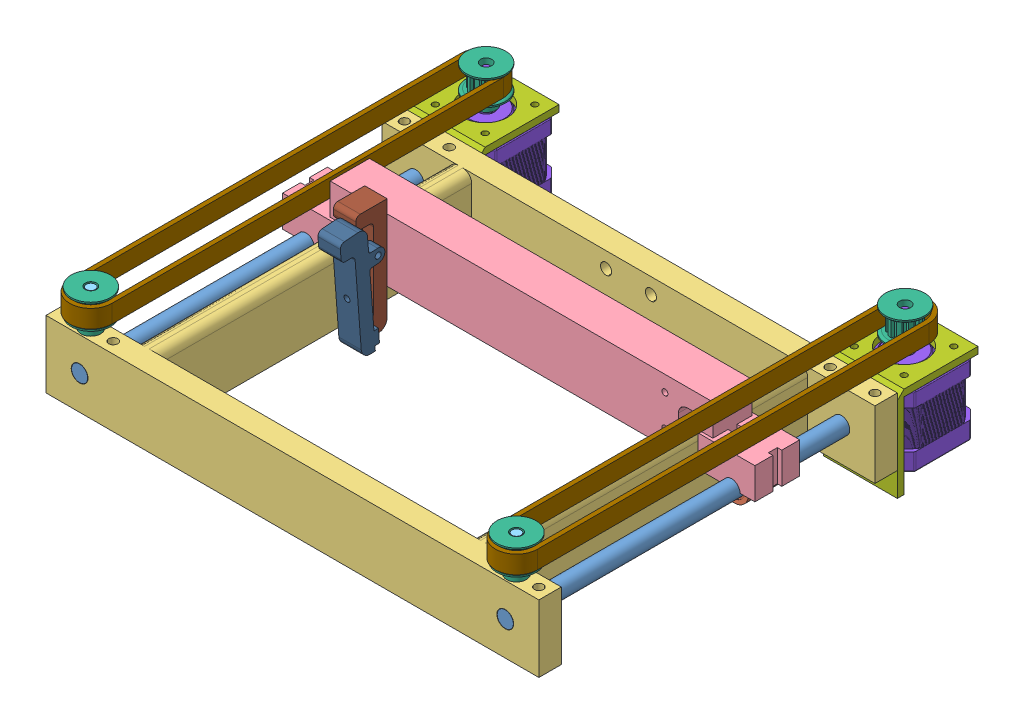
SolidWorks assembly Gantry Assembly, configuration Default. Lengths in mm.
Overall size (280 76.65 262.54).
23 component instances, 11 part files, 39 mates.
Components (placement in the parent):
- 1555T132_Linear Motion Shaft-1: 1555T132_Linear Motion Shaft [1555T132] at (256.3952 90.1087 151.9483) x (0.714788 0.699342 0) z (0 0 1) size (9.53 9.53 203.2)
- 6630K12_Self-Aligning Linear Ball Bearing-1: 6630K12_Self-Aligning Linear Ball Bearing [6630K12] at (256.3952 90.1087 112.5616) size (15.88 15.88 22.23)
- Frame-1: Frame [Default] at (135.7452 70.9617 151.9483) x (0 0 -1) z (1 0 0) size (203.2 38.1 279.4)
- Singular Gantry-1: Singular Gantry [Default] at (135.7452 107.8887 112.5616) size (267.73 35.56 25.4)
- 1555T132_Linear Motion Shaft-2: 1555T132_Linear Motion Shaft [1555T132] at (15.0952 90.1087 151.9483) x (-0.570511 -0.82129 0) z (0 0 -1) size (9.53 9.53 203.2)
- 6630K12_Self-Aligning Linear Ball Bearing-2: 6630K12_Self-Aligning Linear Ball Bearing [6630K12] at (15.0952 90.1087 112.5616) x (0.996009 -0.089256 0) z (0 0 1) size (15.88 15.88 22.23)
- Passive Pulley Axle-1: Passive Pulley Axle [Default] at (256.3952 93.8217 247.1983) x (0.75241 0 -0.658695) z (0.658695 0 0.75241) size (5.08 35.56 5.08)
- Passive Pulley Axle-2: Passive Pulley Axle [Default] at (15.0952 93.8217 247.1983) x (0.614794 0 -0.788687) z (0.788687 0 0.614794) size (5.08 35.56 5.08)
- 6495K744_Timing Belt Pulley-2: 6495K744_Timing Belt Pulley [6495K744] at (256.3952 119.3741 247.1983) x (-0.837169 0 -0.546944) z (0 -1 0) size (22.23 22.23 20.62)
- Mount and Motor-1: Mount and Motor [Default] at (24.9726 -130.2042 -14.5471) x (1 0 0) z (0 1 0) size (42.51 50.31 70.26)
  - Mount (not Blake)-1: Mount (not Blake) [Default] at (-7.9724 -40.1303 235.4559) x (0 0 1) z (0 1 0) size (51.82 41.92 45.73)
  - Stepper Motor-1: Stepper Motor [Default] at (-7.6774 -39.8353 216.7059) size (42.5 46.5 61.75)
- 6495K744_Timing Belt Pulley-3: 6495K744_Timing Belt Pulley [6495K744] at (15.0952 119.3741 247.1983) x (-0.89167 0 -0.452686) z (0 -1 0) size (22.23 22.23 20.62)
- 6495K744_Timing Belt Pulley-9: 6495K744_Timing Belt Pulley [6495K744] at (17.2952 119.3741 25.2883) x (-0.999445 0 -0.033299) z (0 -1 0) size (22.23 22.23 20.62)
- Linear Rod Belt-1: Linear Rod Belt [Default] at (256.3952 127.2354 136.2434) x (0 0 -1) z (-1 0 0) size (245.79 10.16 23.88)
- Linear Rod Belt-2: Linear Rod Belt [Default] at (15.0952 127.2354 136.2434) x (0 0 -1) z (-1 0 0) size (245.79 10.16 23.88)
- Mount and Motor-3: Mount and Motor [Default] at (262.4626 -130.2042 -14.5471) x (1 0 0) z (0 1 0) size (42.51 50.31 70.26)
  - Mount (not Blake)-1: Mount (not Blake) [Default] at (-7.9724 -40.1303 235.4559) x (0 0 1) z (0 1 0) size (51.82 41.92 45.73)
  - Stepper Motor-1: Stepper Motor [Default] at (-7.6774 -39.8353 216.7059) size (42.5 46.5 61.75)
- 6495K744_Timing Belt Pulley-10: 6495K744_Timing Belt Pulley [6495K744] at (254.7852 119.3741 25.2883) x (-0.987813 0 0.155648) z (0 -1 0) size (22.23 22.23 20.62)
- Clip Assembly-1: Clip Assembly [Default] at (100.8747 60.2211 127.9737) x (0 0.02134 0.999772) z (-1 0 0) size (35.62 65.54 20.32)
  - Added Clip Piece-1: Added Clip Piece [Default] at (17.0718 40.185 33.7094) x (0.995308 -0.096757 0) z (0 0 1) size (24.13 63.5 12.7)
  - Attatched Clip Piece-1: Attatched Clip Piece [Default] at (0.3891 41.1725 54.0294) x (-0.999772 0.02134 0) z (0 0 -1) size (17.78 63.5 12.7)
Mates (geometry in assembly coordinates):
- Concentric1: concentric anti-aligned: cylinder of 6630K12_Self-Aligning Linear Ball Bearing-1 through (256.3952 90.1087 123.6741) axis (0 0 -1) radius 7.9375; cylinder of Singular Gantry-1 through (256.3952 90.1087 101.4491) axis (0 0 1) radius 7.9375
- Coincident1: coincident anti-aligned: plane of 6630K12_Self-Aligning Linear Ball Bearing-1 through (256.3952 90.1087 101.4491) normal (0 0 -1); plane of Singular Gantry-1 through (15.0952 90.1087 101.4491) normal (0 0 1)
- Concentric2: concentric aligned: cylinder of 1555T132_Linear Motion Shaft-1 through (256.3952 90.1087 253.5483) axis (0 0 -1) radius 4.7625; cylinder of 6630K12_Self-Aligning Linear Ball Bearing-1 through (256.3952 90.1087 123.6741) axis (0 0 -1) radius 4.8895
- Concentric3: concentric anti-aligned: cylinder of 1555T132_Linear Motion Shaft-1 through (256.3952 90.1087 253.5483) axis (0 0 -1) radius 4.7625; cylinder of Frame-1 through (256.3952 90.1087 -189.6817) axis (0 0 1) radius 4.7625
- Concentric4: concentric aligned: cylinder of Frame-1 through (15.0952 90.1087 -189.6817) axis (0 0 1) radius 4.7625; cylinder of 1555T132_Linear Motion Shaft-2 through (15.0952 90.1087 50.3483) axis (0 0 1) radius 4.7625
- Parallel1: parallel aligned: plane of Frame-1 through (135.7452 109.0617 151.9483) normal (0 1 0); plane of Singular Gantry-1 through (27.2802 125.6687 101.4491) normal (0 1 0)
- Concentric5: concentric anti-aligned: cylinder of Singular Gantry-1 through (15.0952 90.1087 101.4491) axis (0 0 1) radius 7.9375; cylinder of 6630K12_Self-Aligning Linear Ball Bearing-2 through (15.0952 90.1087 123.6741) axis (0 0 -1) radius 7.9375
- Coincident2: coincident anti-aligned: plane of Singular Gantry-1 through (15.0952 90.1087 101.4491) normal (0 0 1); plane of 6630K12_Self-Aligning Linear Ball Bearing-2 through (15.0952 90.1087 101.4491) normal (0 0 -1)
- Concentric6: concentric anti-aligned: cylinder of 1555T132_Linear Motion Shaft-2 through (15.0952 90.1087 50.3483) axis (0 0 1) radius 4.7625; cylinder of 6630K12_Self-Aligning Linear Ball Bearing-2 through (15.0952 90.1087 123.6741) axis (0 0 -1) radius 4.8895
- Coincident3: coincident aligned: plane of Frame-1 through (275.4452 109.0617 253.5483) normal (0 0 1); circle of 1555T132_Linear Motion Shaft-2
- Coincident4: coincident aligned: plane of 1555T132_Linear Motion Shaft-1 through (256.3952 90.1087 253.5483) normal (0 0 1); plane of Frame-1 through (275.4452 109.0617 253.5483) normal (0 0 1)
- Concentric9: concentric aligned: cylinder of Frame-1 through (256.3952 109.0617 247.1983) axis (0 -1 0) radius 2.54; cylinder of Passive Pulley Axle-1 through (256.3952 129.3817 247.1983) axis (0 -1 0) radius 2.54
- Distance1: distance = 20.32 mm aligned: plane of Passive Pulley Axle-1 through (256.3952 129.3817 247.1983) normal (0 1 0); plane of Frame-1 through (135.7452 109.0617 151.9483) normal (0 1 0)
- Concentric10: concentric aligned: cylinder of Frame-1 through (15.0952 109.0617 247.1983) axis (0 -1 0) radius 2.54; cylinder of Passive Pulley Axle-2 through (15.0952 129.3817 247.1983) axis (0 -1 0) radius 2.54
- Distance2: distance = 20.32 mm aligned: plane of Passive Pulley Axle-2 through (15.0952 129.3817 247.1983) normal (0 1 0); plane of Frame-1 through (135.7452 109.0617 151.9483) normal (0 1 0)
- Coincident8: coincident anti-aligned: plane of Frame-1 through (224.6452 109.0617 50.3483) normal (0 0 -1); plane of Mount and Motor-1/Mount (not Blake)-1 through (17.0002 105.2517 50.3483) normal (0 0 1)
- Concentric14: concentric aligned: cylinder of Passive Pulley Axle-1 through (256.3952 129.3817 247.1983) axis (0 -1 0) radius 2.54; cylinder of 6495K744_Timing Belt Pulley-2 through (256.3952 109.0617 247.1983) axis (0 -1 0) radius 3.175
- Coincident9: coincident anti-aligned: plane of Frame-1 through (135.7452 109.0617 151.9483) normal (0 1 0); plane of 6495K744_Timing Belt Pulley-2 through (254.6587 109.0617 249.8563) normal (0 -1 0)
- Concentric15: concentric aligned: cylinder of Passive Pulley Axle-2 through (15.0952 129.3817 247.1983) axis (0 -1 0) radius 2.54; cylinder of 6495K744_Timing Belt Pulley-3 through (15.0952 109.0617 247.1983) axis (0 -1 0) radius 3.175
- Coincident10: coincident anti-aligned: plane of Frame-1 through (135.7452 109.0617 151.9483) normal (0 1 0); plane of 6495K744_Timing Belt Pulley-3 through (13.658 109.0617 250.0293) normal (0 -1 0)
- Concentric18: concentric aligned: cylinder of Mount and Motor-1/Stepper Motor-1 through (17.2952 127.5017 25.2883) axis (0 -1 0) radius 2.5; cylinder of 6495K744_Timing Belt Pulley-9 through (17.2952 109.0617 25.2883) axis (0 -1 0) radius 3.175
- Coincident13: coincident anti-aligned: plane of Mount and Motor-1/Mount (not Blake)-1 through (17.0002 109.0617 25.5833) normal (0 1 0); plane of 6495K744_Timing Belt Pulley-9 through (17.1895 109.0617 28.4615) normal (0 -1 0)
- Coincident14: coincident anti-aligned: plane of Frame-1 through (224.6452 109.0617 50.3483) normal (0 0 -1); plane of Mount and Motor-1/Mount (not Blake)-1 through (17.0002 105.2517 50.3483) normal (0 0 1)
- Parallel2: parallel aligned: plane of Frame-1 through (135.7452 70.9617 151.9483) normal (0 -1 0); plane of Mount and Motor-1/Mount (not Blake)-1 through (37.9552 57.2457 50.3483) normal (0 -1 0)
- Concentric20: concentric anti-aligned: circle of 6495K744_Timing Belt Pulley-2; cylinder of Linear Rod Belt-1 through (256.3952 117.0754 247.1983) axis (0 1 0) radius 9.398
- Concentric22: concentric anti-aligned: circle of 6495K744_Timing Belt Pulley-3; cylinder of Linear Rod Belt-2 through (15.0952 117.0754 247.1983) axis (0 1 0) radius 9.398
- Coincident15: coincident anti-aligned: plane of 6495K744_Timing Belt Pulley-3 through (10.8064 117.0754 255.6461) normal (0 1 0); plane of Linear Rod Belt-2 through (15.0952 117.0754 247.1983) normal (0 -1 0)
- Coincident16: coincident anti-aligned: plane of 6495K744_Timing Belt Pulley-2 through (251.2134 117.0754 255.1298) normal (0 1 0); plane of Linear Rod Belt-1 through (256.3952 117.0754 247.1983) normal (0 -1 0)
- Coincident17: coincident aligned: plane of Frame-1 through (-3.9548 109.0617 63.0483) normal (-1 0 0); plane of Mount and Motor-1/Mount (not Blake)-1 through (-3.9548 109.0617 4.6283) normal (-1 0 0)
- Coincident19: coincident aligned: plane of Frame-1 through (135.7452 109.0617 151.9483) normal (0 1 0); plane of Mount and Motor-1/Mount (not Blake)-1 through (17.0002 109.0617 25.5833) normal (0 1 0)
- Parallel3: parallel aligned: plane of Singular Gantry-1 through (1.8802 107.8887 101.4491) normal (-1 0 0); plane of Linear Rod Belt-2 through (3.1572 117.0754 247.1983) normal (-1 0 0)
- Parallel5: parallel aligned: plane of Frame-1 through (275.4452 109.0617 63.0483) normal (1 0 0); plane of Linear Rod Belt-1 through (268.3332 117.0754 247.1983) normal (1 0 0)
- Coincident25: coincident anti-aligned: plane of Frame-1 through (224.6452 109.0617 50.3483) normal (0 0 -1); plane of Mount and Motor-3/Mount (not Blake)-1 through (254.4902 105.2517 50.3483) normal (0 0 1)
- Coincident26: coincident aligned: plane of Frame-1 through (275.4452 109.0617 63.0483) normal (1 0 0); plane of Mount and Motor-3/Mount (not Blake)-1 through (275.4452 109.0617 4.6283) normal (1 0 0)
- Coincident27: coincident aligned: plane of Frame-1 through (135.7452 109.0617 151.9483) normal (0 1 0); plane of Mount and Motor-3/Mount (not Blake)-1 through (254.4902 109.0617 25.5833) normal (0 1 0)
- Concentric23: concentric aligned: cylinder of Mount and Motor-3/Stepper Motor-1 through (254.7852 127.5017 25.2883) axis (0 -1 0) radius 2.5; cylinder of 6495K744_Timing Belt Pulley-10 through (254.7852 109.0617 25.2883) axis (0 -1 0) radius 3.175
- Coincident28: coincident anti-aligned: plane of Mount and Motor-3/Mount (not Blake)-1 through (254.4902 109.0617 25.5833) normal (0 1 0); plane of 6495K744_Timing Belt Pulley-10 through (255.2794 109.0617 28.4246) normal (0 -1 0)
- Coincident29: coincident anti-aligned: plane of Singular Gantry-1 through (256.3952 90.1087 123.6741) normal (0 0 1); plane of Clip Assembly-1/Attatched Clip Piece-1 through (59.5452 133.1425 123.6741) normal (0 0 -1)
- Coincident30: coincident anti-aligned: plane of Frame-1 through (46.8452 109.0617 240.8483) normal (1 0 0); plane of Clip Assembly-1/Attatched Clip Piece-1 through (46.8452 74.7225 128.7541) normal (-1 0 0)
